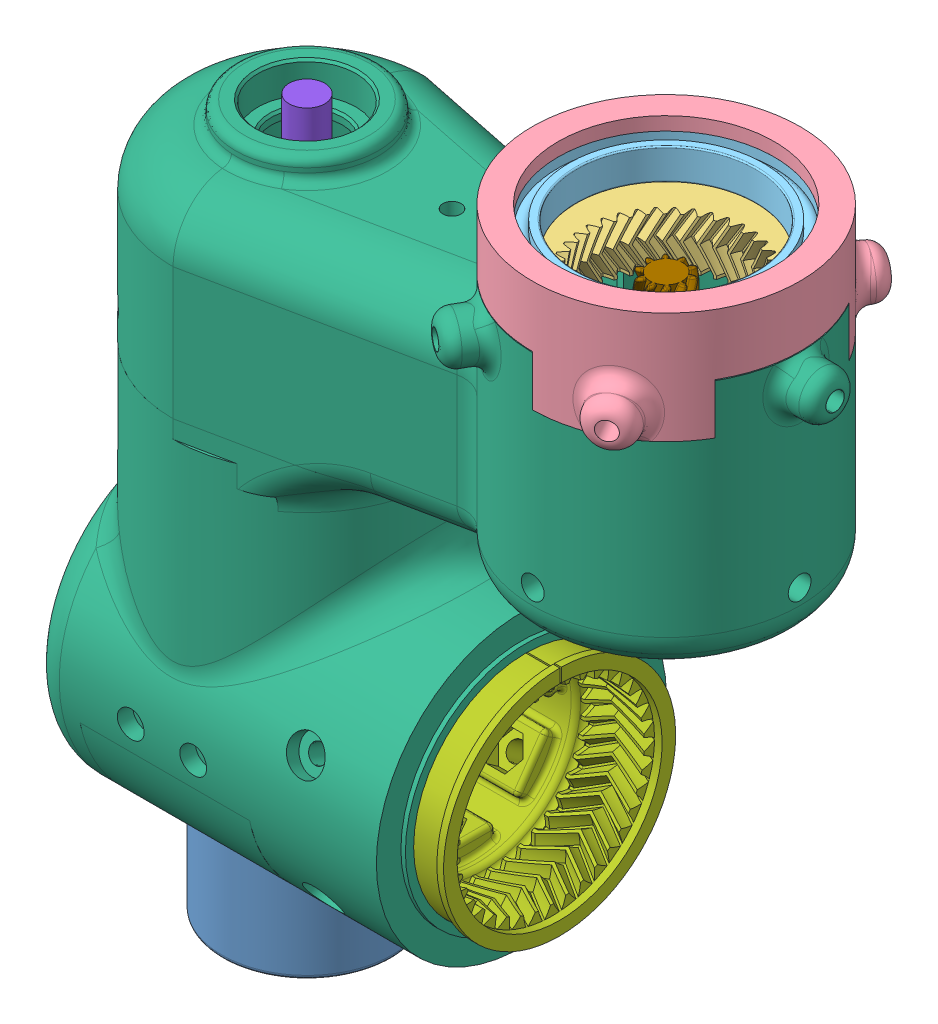
SolidWorks assembly A6 Assembly, configuration Default. Lengths in mm.
Overall size (157.9 177.54 88.85).
9 component instances, 9 part files, 30 mates.
Components (placement in the parent):
- Encoder600PR-1: Encoder600PR [Default] at (3.921 38.6161 35.8814) x (0.31767 0 -0.948201) z (0.948201 0 0.31767) size (38 53 38)
- Propdrive v2 3536-910kv-1: Propdrive v2 3536-910kv [Default] at (3.921 99.3161 35.8814) x (0.262612 0 -0.964901) z (0.964901 0 0.262612) size (35.77 56 35.77)
- A6D2 - Output Ring-1: A6D2 - Output Ring [Default] at (62.5859 241.5311 -68.312) x (0.372467 0 0.928046) z (0 1 0) size (51.9 51.9 11.34)
- A6D3 - Output Bracket-1: A6D3 - Output Bracket [Default] at (84.421 191.1961 35.8814) x (0.866025 0 0.5) z (-0.5 0 0.866025) size (62.86 29.34 66.3)
- radial ball bearing_68_iso-6: radial ball bearing_68_iso [ISO 15 RBB - 1840 - 32,SI,NC,32_68] at (84.421 209.6561 35.8814) x (0 1 0) z (-0.843815 0 0.536635) size (7 52 52)
- A6D1 - Main-1: A6D1 - Main [Default] at (12.946 55.6161 35.8814) x (-1 0 0) z (0 0 -1) size (149.14 147.19 68.51)
- A6 - Input Ring (alt-50)-1: A6 - Input Ring (alt-50) [Default] at (60.2543 88.1161 35.8814) x (0 0 -1) z (1 0 0) size (52 52 32.37)
- pulley_24T-1: pulley_24T [Default] at (3.921 174.3161 35.8814) x (0.675233 0 -0.737605) z (0 -1 0) size (25.16 25.16 56)
- pulley_24T_receiver-1: pulley_24T_receiver [Default] at (84.421 159.3161 35.8814) x (-0.910803 0 -0.412841) z (0 1 0) size (25.16 25.16 61.72)
Mates (geometry in assembly coordinates):
- Coincident2: coincident: plane of ? through (19.1611 141.1234 2.3906) normal (0.99916 0 0.040976); plane of ? through (19.1396 144.9373 2.9162) normal (-0.99916 0 -0.040976)
- Concentric3: concentric: cylinder of ? through (19.1611 141.1234 2.3906) axis (0.99916 0 0.040976) radius 7.5; cylinder of ? through (1.0389 141.1234 1.6474) axis (0.99916 0 0.040976) radius 7
- Concentric4: concentric: cylinder of ? through (1.0389 141.1234 1.6474) axis (0.99916 0 0.040976) radius 2.5; cylinder of ? through (60.8761 141.1234 4.1014) axis (0.99916 0 0.040976) radius 4.25
- Coincident3: coincident: plane of ? through (24.1418 143.7981 2.9641) normal (0.99916 0 0.040976); plane of ? through (24.1569 145.3734 2.5955) normal (-0.99916 0 -0.040976)
- Concentric5: concentric: cylinder of ? through (21.47 54.3511 -60.0353) axis (0 -0.34202 0.939693) radius 2.05; cylinder of ? through (21.47 43.5031 -30.2308) axis (0 -0.34202 0.939693) radius 2.05
- Concentric6: concentric: cylinder of ? through (-6 32.5 0) axis (1 0 0) radius 25.15; cylinder of ? through (31.584 32.5 0) axis (1 0 0) radius 25.1
- Concentric7: concentric: cylinder of assembly through (-8.5 130 0) axis (0 -1 0) radius 30; cylinder of ?; cylinder of Encoder600PR-1 through (3.921 73.6161 35.8814) axis (0 -1 0) radius 19
- Concentric8: concentric aligned: cylinder of Encoder600PR-1 through (3.921 73.6161 35.8814) axis (0 -1 0) radius 19; cylinder of Propdrive v2 3536-910kv-1 through (3.921 126.3161 35.8814) axis (0 -1 0) radius 17.5
- Concentric9: concentric: cylinder of ? through (-6 146.33 0) axis (0 -1 0) radius 26; cylinder of ? through (-6 199.9078 0) axis (0 1 0) radius 26
- Coincident4: coincident: plane of assembly through (-8.5 130 0) normal (0 1 0); plane of ?; plane of A6D2 - Output Ring-1 through (84.421 191.1961 35.8814) normal (0 -1 0)
- Parallel1: parallel: cylinder of assembly through (-45.0741 135.665 -21.1161) axis (0.866025 0 0.5) radius 2.05; cylinder of ?; cylinder of A6D2 - Output Ring-1 through (74.6373 196.8627 18.4952) axis (-0.490414 0 -0.871489) radius 2.05
- Concentric11: concentric: cylinder of assembly through (-8.5 130 0) axis (0 -1 0) radius 30; cylinder of ?; cylinder of A6D2 - Output Ring-1 through (84.421 117.7984 35.8814) axis (0 1 0) radius 25.95
- Distance1: distance = 62.7 mm aligned: plane of Propdrive v2 3536-910kv-1 through (3.921 136.3161 35.8814) normal (0 1 0); plane of Encoder600PR-1 through (3.921 73.6161 35.8814) normal (0 1 0)
- Concentric16: concentric: cylinder of ? through (27.7798 85.6961 4.5833) axis (1 0 0) radius 25.1; cylinder of A6D1 - Main-1 through (10.971 88.1161 35.8814) axis (1 0 0) radius 25.15
- Coincident6: coincident anti-aligned: plane of Encoder600PR-1 through (3.921 73.6161 35.8814) normal (0 1 0); plane of A6D1_new-1 through (12.946 73.6161 35.8814) normal (0 -1 0)
- Concentric18: concentric aligned: cylinder of Encoder600PR-1 through (3.921 78.6161 35.8814) axis (0 -1 0) radius 10; cylinder of A6D1_new-1 through (3.921 81.6161 35.8814) axis (0 -1 0) radius 12
- Parallel2: parallel anti-aligned: plane of Propdrive v2 3536-910kv-1 through (3.921 136.3161 35.8814) normal (0 1 0); plane of A6D1_new-1 through (12.946 136.3161 35.8814) normal (0 -1 0)
- Distance3: distance = 0.5 mm: cylinder of ? through (17.6735 96.6992 -25.6475) axis (0 -0.34202 0.939693) radius 2.05; cylinder of A6D1 - Main-1 through (34.171 105.7068 -12.4487) axis (0 -0.34202 0.939693) radius 2.05
- Concentric26: concentric aligned: cylinder of A6D1_new-1 through (10.971 88.1161 35.8814) axis (1 0 0) radius 25.15; cylinder of A6D1 Ring From A5_50version-1 through (44.671 88.1161 35.8814) axis (1 0 0) radius 25.1
- Concentric27: concentric aligned: cylinder of A6D1_new-1 through (34.171 105.7068 -12.4487) axis (0 -0.34202 0.939693) radius 2.05; cylinder of A6D1 Ring From A5_50version-1 through (34.171 99.1192 5.6506) axis (0 -0.34202 0.939693) radius 2.05
- Coincident7: coincident anti-aligned: plane of A6D3-1 through (84.421 213.1561 35.8814) normal (0 -1 0); plane of radial ball bearing_68_iso-6 through (70.6295 213.1561 14.1954) normal (0 1 0)
- Concentric28: concentric anti-aligned: cylinder of A6D3-1 through (84.421 202.5261 35.8814) axis (0 -1 0) radius 30; cylinder of radial ball bearing_68_iso-6 through (84.421 189.0186 35.8814) axis (0 1 0) radius 26
- Coincident8: coincident aligned: plane of A6D2 Ring To End-1 through (84.421 191.1961 35.8814) normal (0 -1 0); plane of A6D3-1 through (84.421 191.1961 35.8814) normal (0 -1 0)
- Concentric29: concentric anti-aligned: cylinder of A6D2 Ring To End-1 through (84.421 117.7984 35.8814) axis (0 1 0) radius 25.95; cylinder of A6D3-1 through (84.421 202.5261 35.8814) axis (0 -1 0) radius 30
- Coincident9: coincident anti-aligned: plane of A6D2 Ring To End-1 through (84.421 191.1961 35.8814) normal (0 -1 0); plane of A6D1_new-1 through (84.421 191.1961 35.8814) normal (0 1 0)
- Concentric30: concentric anti-aligned: cylinder of A6D3-1 through (84.421 202.5261 35.8814) axis (0 -1 0) radius 30; cylinder of A6D1_new-1 through (84.421 55.6151 35.8814) axis (0 1 0) radius 30
- Coincident10: coincident anti-aligned: plane of A6D3-1 through (84.421 202.5261 35.8814) normal (0.5 0 0.866025); plane of A6D1_new-1 through (110.4018 202.3261 20.8814) normal (-0.5 0 -0.866025)
- Distance4: distance = 1 mm anti-aligned: plane of A6D1_new-1 through (12.946 140.3161 35.8814) normal (0 1 0); plane of pulley_24T-1 through (3.921 141.3161 35.8814) normal (0 -1 0)
- Concentric32: concentric aligned: cylinder of A6D1_new-1 through (84.421 147.1961 35.8814) axis (0 -1 0) radius 11; cylinder of pulley_24T_receiver-1 through (84.421 203.6298 35.8814) axis (0 -1 0) radius 4
- Coincident12: coincident: line of pulley_24T-1 through (0.1329 159.3161 23.8873) axis (0.962902 0 -0.269853); plane of pulley_24T_receiver-1 through (84.421 159.3161 35.8814) normal (0 -1 0)
